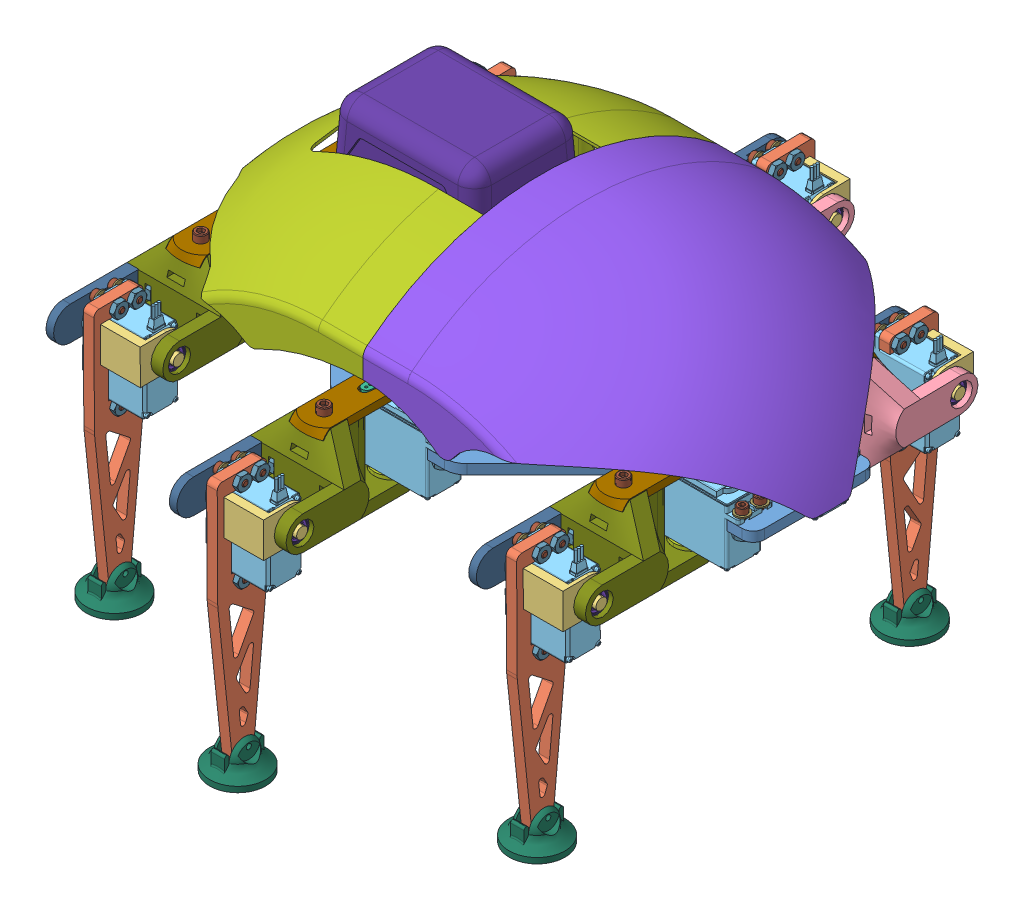
SolidWorks assembly Hexapod_NewBody, configuration Défaut. Lengths in mm.
Overall size (338.69 233.7 350.76).
398 component instances, 26 part files, 150 mates.
Components (placement in the parent):
- Body_V2-5: Body_V2 [Default] at (-310 -5.6 15) x (1 0 0) z (0 1 0) size (310 170 5.6)
- Leg_(Straight_Foot)-6: Leg_(Straight_Foot) [Default] at (-54.94 -26.67 -0.094) size (71.12 162.26 125.96)
  - Foot_(Straight)-1: Foot_(Straight) [Default] at (4.9357 4.6699 -91.3683) x (0.014203 -0.004158 0.99989) z (-0.999899 0 0.014203) size (28 145.4 6)
  - bearing_mount_foot-1: bearing_mount_foot [Default] at (4.8169 16.6428 -99.7277) x (-0.014203 0.004158 -0.99989) z (0.999899 0 -0.014203) size (25 20 29.5)
  - Joint-1: Joint [Défaut] at (35.768 26.4662 -54.7315) x (-0.014203 0 -0.999899) z (0 1 0) size (96.52 53.26 53.26)
  - hs-422-2: hs-422 [Défaut] at (5.1023 6.6131 -77.4551) x (-0.014203 0.004158 -0.99989) z (0.000059 0.999991 0.004158) size (19.81 42.09 58.23)
  - hs-422-3: hs-422 [Défaut] at (19.939 20.701 -19.812) x (0 0 1) z (-1 0 0) size (19.81 42.09 58.23)
  - hs-422_horn_straight-1: hs-422_horn_straight [Default] at (-16.9088 16.9412 -87.0065) x (0.014203 0 0.999899) z (0 1 0) size (33.93 4.93 8.79)
  - hs-422_horn_straight-2: hs-422_horn_straight [Default] at (9.652 42.5743 -9.906) x (-0.014203 0 -0.999899) z (-0.999899 0 0.014203) size (33.93 4.93 8.79)
  - Bearing_mount_leg-1: Bearing_mount_leg [Default] at (9.652 21 2.594) x (0 0 1) z (0 -1 0) size (35 20 30)
  - Bearing-1: Bearing [Default] at (9.652 -6.7498 -9.906) x (0.84763 0 0.530588) z (-0.530588 0 0.84763) size (13.87 4.75 13.87)
  - Bearing-2: Bearing [Default] at (32.2403 16.9412 -87.7047) x (0.007588 -0.845349 0.534161) z (-0.012007 -0.534214 -0.845264) size (13.87 4.75 13.87)
  - Joint_attachment_leg-1: Joint_attachment_leg [Défaut] at (35.768 26.4662 -54.7315) x (-0.014203 0 -0.999899) z (0 1 0) size (74.32 19.07 4.32)
  - Joint_attachment_foot-1: Joint_attachment_foot [Défaut] at (35.768 26.4662 -54.7315) x (-0.014203 0 -0.999899) z (0 1 0) size (64.08 6.7 19.07)
  - socket_1_2_6-32_with_washer-1: socket_1_2_6-32_with_washer [Défaut] at (43.4196 -14.698 -83.8589) x (0.999899 0 -0.014203) z (0.012271 -0.503597 0.863852) size (16.21 7.92 7.92)
    - socket head cap screw_ai-1: socket head cap screw_ai [HX-SHCS 0.138-32x0.5x0.5-N] at (-51.206 -1.62 2.0257) size (16.21 5.74 5.74)
    - flat washer type b narrow_ai-1: flat washer type b narrow_ai [Narrow FW 0.138] at (-46.888 -1.62 2.0257) size (0.81 7.92 7.92)
  - socket_1_2_6-32_with_washer-2: socket_1_2_6-32_with_washer [Défaut] at (43.2654 -19.0943 -94.7118) x (0.999899 0 -0.014203) z (0.000059 0.999991 0.004158) size (16.21 7.92 7.92)
    - socket head cap screw_ai-1: socket head cap screw_ai [HX-SHCS 0.138-32x0.5x0.5-N] at (-51.206 -1.62 2.0257) size (16.21 5.74 5.74)
    - flat washer type b narrow_ai-1: flat washer type b narrow_ai [Narrow FW 0.138] at (-46.888 -1.62 2.0257) size (0.81 7.92 7.92)
  - socket_1_2_6-32_with_washer-3: socket_1_2_6-32_with_washer [Défaut] at (43.4489 27.9623 -81.7931) x (0.999899 0 -0.014203) z (-0.012271 0.503597 -0.863852) size (16.21 7.92 7.92)
    - socket head cap screw_ai-1: socket head cap screw_ai [HX-SHCS 0.138-32x0.5x0.5-N] at (-51.206 -1.62 2.0257) size (16.21 5.74 5.74)
    - flat washer type b narrow_ai-1: flat washer type b narrow_ai [Narrow FW 0.138] at (-46.888 -1.62 2.0257) size (0.81 7.92 7.92)
  - socket_1_2_6-32_with_washer-4: socket_1_2_6-32_with_washer [Défaut] at (43.3046 28.0045 -91.952) x (0.999899 0 -0.014203) z (-0.012271 0.503597 -0.863852) size (16.21 7.92 7.92)
    - socket head cap screw_ai-1: socket head cap screw_ai [HX-SHCS 0.138-32x0.5x0.5-N] at (-51.206 -1.62 2.0257) size (16.21 5.74 5.74)
    - flat washer type b narrow_ai-1: flat washer type b narrow_ai [Narrow FW 0.138] at (-46.888 -1.62 2.0257) size (0.81 7.92 7.92)
  - socket button head cap screw_ai-2: socket button head cap screw_ai [SBHCSCREW 0.112-40x0.25-HX-N] at (-19.9057 16.9412 -86.964) x (0.999899 0 -0.014203) z (-0.007102 0.866025 -0.49995) size (7.85 5.41 5.41)
  - socket button head cap screw_ai-3: socket button head cap screw_ai [SBHCSCREW 0.112-40x0.25-HX-N] at (9.652 45.5715 -9.906) x (0 -1 0) z (0.87304 0 0.487649) size (7.85 5.41 5.41)
  - machine screw nut hex_ai-7: machine screw nut hex_ai [MSHXNUT 0.138-32-D-N] at (5.0634 -17.1176 -82.3797) x (0.01233 0.496395 0.868009) z (-0.999899 0 0.014203) size (7.92 9.15 2.9)
  - machine screw nut hex_ai-8: machine screw nut hex_ai [MSHXNUT 0.138-32-D-N] at (4.9191 -17.0754 -92.5386) x (-0.012271 0.503597 -0.863852) z (-0.999899 0 0.014203) size (7.92 9.15 2.9)
  - machine screw nut hex_ai-9: machine screw nut hex_ai [MSHXNUT 0.138-32-D-N] at (5.0662 30.382 -82.1822) x (0.000059 0.999991 0.004158) z (-0.999899 0 0.014203) size (7.92 9.15 2.9)
  - machine screw nut hex_ai-10: machine screw nut hex_ai [MSHXNUT 0.138-32-D-N] at (4.9219 30.4242 -92.3411) x (0.000059 0.999991 0.004158) z (-0.999899 0 0.014203) size (7.92 9.15 2.9)
  - socket head cap screw_ai-1: socket head cap screw_ai [HX-SHCS 0.164-32x0.5x0.5-N] at (9.1052 47.8568 -48.4) x (0 -1 0) z (0.014203 0 0.999899) size (16.87 6.86 6.86)
  - socket head cap screw_ai-2: socket head cap screw_ai [HX-SHCS 0.164-32x0.5x0.5-N] at (-21.967 16.9412 -59.205) x (0.999899 0 -0.014203) z (0.014203 0 0.999899) size (16.87 6.86 6.86)
  - machine screw nut hex_ai-11: machine screw nut hex_ai [MSHXNUT 0.164-32-D-N] at (9.1052 33.127 -48.4) x (0.87304 0 0.487649) z (0 1 0) size (8.74 10.09 3.3)
  - machine screw nut hex_ai-12: machine screw nut hex_ai [MSHXNUT 0.164-32-D-N] at (-7.2387 16.9412 -59.4142) x (0.014203 0 0.999899) z (-0.999899 0 0.014203) size (8.74 10.09 3.3)
  - socket head cap screw_ai-3: socket head cap screw_ai [HX-SHCS 0.112-40x0.5x0.5-N] at (-4.0273 11.7048 -99.6226) x (0.999899 0 -0.014203) z (0.014203 -0.004158 0.99989) size (15.54 4.65 4.65)
  - socket head cap screw_ai-4: socket head cap screw_ai [HX-SHCS 0.112-40x0.5x0.5-N] at (-4.0267 21.7048 -99.5811) x (0.999899 0 -0.014203) z (-0.014203 0.004158 -0.99989) size (15.54 4.65 4.65)
  - socket_1_2_6-32_with_washer-5: socket_1_2_6-32_with_washer [Défaut] at (-3.4199 -17.7034 -7.3903) x (0 -1 0) z (0.5 0 0.866025) size (16.21 7.92 7.92)
    - socket head cap screw_ai-1: socket head cap screw_ai [HX-SHCS 0.138-32x0.5x0.5-N] at (-51.206 -1.62 2.0257) size (16.21 5.74 5.74)
    - flat washer type b narrow_ai-1: flat washer type b narrow_ai [Narrow FW 0.138] at (-46.888 -1.62 2.0257) size (0.81 7.92 7.92)
  - socket_1_2_6-32_with_washer-6: socket_1_2_6-32_with_washer [Défaut] at (44.0781 -17.7034 -17.5503) x (0 -1 0) z (0.5 0 0.866025) size (16.21 7.92 7.92)
    - socket head cap screw_ai-1: socket head cap screw_ai [HX-SHCS 0.138-32x0.5x0.5-N] at (-51.206 -1.62 2.0257) size (16.21 5.74 5.74)
    - flat washer type b narrow_ai-1: flat washer type b narrow_ai [Narrow FW 0.138] at (-46.888 -1.62 2.0257) size (0.81 7.92 7.92)
  - socket_1_2_6-32_with_washer-7: socket_1_2_6-32_with_washer [Défaut] at (-3.4199 -17.7034 -17.5503) x (0 -1 0) z (0.5 0 0.866025) size (16.21 7.92 7.92)
    - socket head cap screw_ai-1: socket head cap screw_ai [HX-SHCS 0.138-32x0.5x0.5-N] at (-51.206 -1.62 2.0257) size (16.21 5.74 5.74)
    - flat washer type b narrow_ai-1: flat washer type b narrow_ai [Narrow FW 0.138] at (-46.888 -1.62 2.0257) size (0.81 7.92 7.92)
  - socket_1_2_6-32_with_washer-8: socket_1_2_6-32_with_washer [Défaut] at (44.0781 -17.7034 -7.3903) x (0 -1 0) z (0.5 0 0.866025) size (16.21 7.92 7.92)
    - socket head cap screw_ai-1: socket head cap screw_ai [HX-SHCS 0.138-32x0.5x0.5-N] at (-51.206 -1.62 2.0257) size (16.21 5.74 5.74)
    - flat washer type b narrow_ai-1: flat washer type b narrow_ai [Narrow FW 0.138] at (-46.888 -1.62 2.0257) size (0.81 7.92 7.92)
  - Slippers-1: Slippers [Default] at (1.9298 -111.2299 -91.7597) x (0.999899 0 -0.014203) z (0.014203 0 0.999899) size (35.48 18.25 37.71)
- Leg_(Straight_Foot)-7: Leg_(Straight_Foot) [Default] at (-294.94 -26.67 -0.094) size (71.12 162.26 125.96)
  - Foot_(Straight)-1: Foot_(Straight) [Default] at (4.9357 4.6699 -91.3683) x (0.014203 -0.004158 0.99989) z (-0.999899 0 0.014203) size (28 145.4 6)
  - bearing_mount_foot-1: bearing_mount_foot [Default] at (4.8169 16.6428 -99.7277) x (-0.014203 0.004158 -0.99989) z (0.999899 0 -0.014203) size (25 20 29.5)
  - Joint-1: Joint [Défaut] at (35.768 26.4662 -54.7315) x (-0.014203 0 -0.999899) z (0 1 0) size (96.52 53.26 53.26)
  - hs-422-2: hs-422 [Défaut] at (5.1023 6.6131 -77.4551) x (-0.014203 0.004158 -0.99989) z (0.000059 0.999991 0.004158) size (19.81 42.09 58.23)
  - hs-422-3: hs-422 [Défaut] at (19.939 20.701 -19.812) x (0 0 1) z (-1 0 0) size (19.81 42.09 58.23)
  - hs-422_horn_straight-1: hs-422_horn_straight [Default] at (-16.9088 16.9412 -87.0065) x (0.014203 0 0.999899) z (0 1 0) size (33.93 4.93 8.79)
  - hs-422_horn_straight-2: hs-422_horn_straight [Default] at (9.652 42.5743 -9.906) x (-0.014203 0 -0.999899) z (-0.999899 0 0.014203) size (33.93 4.93 8.79)
  - Bearing_mount_leg-1: Bearing_mount_leg [Default] at (9.652 21 2.594) x (0 0 1) z (0 -1 0) size (35 20 30)
  - Bearing-1: Bearing [Default] at (9.652 -6.7498 -9.906) x (0.84763 0 0.530588) z (-0.530588 0 0.84763) size (13.87 4.75 13.87)
  - Bearing-2: Bearing [Default] at (32.2403 16.9412 -87.7047) x (0.007588 -0.845349 0.534161) z (-0.012007 -0.534214 -0.845264) size (13.87 4.75 13.87)
  - Joint_attachment_leg-1: Joint_attachment_leg [Défaut] at (35.768 26.4662 -54.7315) x (-0.014203 0 -0.999899) z (0 1 0) size (74.32 19.07 4.32)
  - Joint_attachment_foot-1: Joint_attachment_foot [Défaut] at (35.768 26.4662 -54.7315) x (-0.014203 0 -0.999899) z (0 1 0) size (64.08 6.7 19.07)
  - socket_1_2_6-32_with_washer-1: socket_1_2_6-32_with_washer [Défaut] at (43.4196 -14.698 -83.8589) x (0.999899 0 -0.014203) z (0.012271 -0.503597 0.863852) size (16.21 7.92 7.92)
    - socket head cap screw_ai-1: socket head cap screw_ai [HX-SHCS 0.138-32x0.5x0.5-N] at (-51.206 -1.62 2.0257) size (16.21 5.74 5.74)
    - flat washer type b narrow_ai-1: flat washer type b narrow_ai [Narrow FW 0.138] at (-46.888 -1.62 2.0257) size (0.81 7.92 7.92)
  - socket_1_2_6-32_with_washer-2: socket_1_2_6-32_with_washer [Défaut] at (43.2654 -19.0943 -94.7118) x (0.999899 0 -0.014203) z (0.000059 0.999991 0.004158) size (16.21 7.92 7.92)
    - socket head cap screw_ai-1: socket head cap screw_ai [HX-SHCS 0.138-32x0.5x0.5-N] at (-51.206 -1.62 2.0257) size (16.21 5.74 5.74)
    - flat washer type b narrow_ai-1: flat washer type b narrow_ai [Narrow FW 0.138] at (-46.888 -1.62 2.0257) size (0.81 7.92 7.92)
  - socket_1_2_6-32_with_washer-3: socket_1_2_6-32_with_washer [Défaut] at (43.4489 27.9623 -81.7931) x (0.999899 0 -0.014203) z (-0.012271 0.503597 -0.863852) size (16.21 7.92 7.92)
    - socket head cap screw_ai-1: socket head cap screw_ai [HX-SHCS 0.138-32x0.5x0.5-N] at (-51.206 -1.62 2.0257) size (16.21 5.74 5.74)
    - flat washer type b narrow_ai-1: flat washer type b narrow_ai [Narrow FW 0.138] at (-46.888 -1.62 2.0257) size (0.81 7.92 7.92)
  - socket_1_2_6-32_with_washer-4: socket_1_2_6-32_with_washer [Défaut] at (43.3046 28.0045 -91.952) x (0.999899 0 -0.014203) z (-0.012271 0.503597 -0.863852) size (16.21 7.92 7.92)
    - socket head cap screw_ai-1: socket head cap screw_ai [HX-SHCS 0.138-32x0.5x0.5-N] at (-51.206 -1.62 2.0257) size (16.21 5.74 5.74)
    - flat washer type b narrow_ai-1: flat washer type b narrow_ai [Narrow FW 0.138] at (-46.888 -1.62 2.0257) size (0.81 7.92 7.92)
  - socket button head cap screw_ai-2: socket button head cap screw_ai [SBHCSCREW 0.112-40x0.25-HX-N] at (-19.9057 16.9412 -86.964) x (0.999899 0 -0.014203) z (-0.007102 0.866025 -0.49995) size (7.85 5.41 5.41)
  - socket button head cap screw_ai-3: socket button head cap screw_ai [SBHCSCREW 0.112-40x0.25-HX-N] at (9.652 45.5715 -9.906) x (0 -1 0) z (0.87304 0 0.487649) size (7.85 5.41 5.41)
  - machine screw nut hex_ai-7: machine screw nut hex_ai [MSHXNUT 0.138-32-D-N] at (5.0634 -17.1176 -82.3797) x (0.01233 0.496395 0.868009) z (-0.999899 0 0.014203) size (7.92 9.15 2.9)
  - machine screw nut hex_ai-8: machine screw nut hex_ai [MSHXNUT 0.138-32-D-N] at (4.9191 -17.0754 -92.5386) x (-0.012271 0.503597 -0.863852) z (-0.999899 0 0.014203) size (7.92 9.15 2.9)
  - machine screw nut hex_ai-9: machine screw nut hex_ai [MSHXNUT 0.138-32-D-N] at (5.0662 30.382 -82.1822) x (0.000059 0.999991 0.004158) z (-0.999899 0 0.014203) size (7.92 9.15 2.9)
  - machine screw nut hex_ai-10: machine screw nut hex_ai [MSHXNUT 0.138-32-D-N] at (4.9219 30.4242 -92.3411) x (0.000059 0.999991 0.004158) z (-0.999899 0 0.014203) size (7.92 9.15 2.9)
  - socket head cap screw_ai-1: socket head cap screw_ai [HX-SHCS 0.164-32x0.5x0.5-N] at (9.1052 47.8568 -48.4) x (0 -1 0) z (0.014203 0 0.999899) size (16.87 6.86 6.86)
  - socket head cap screw_ai-2: socket head cap screw_ai [HX-SHCS 0.164-32x0.5x0.5-N] at (-21.967 16.9412 -59.205) x (0.999899 0 -0.014203) z (0.014203 0 0.999899) size (16.87 6.86 6.86)
  - machine screw nut hex_ai-11: machine screw nut hex_ai [MSHXNUT 0.164-32-D-N] at (9.1052 33.127 -48.4) x (0.87304 0 0.487649) z (0 1 0) size (8.74 10.09 3.3)
  - machine screw nut hex_ai-12: machine screw nut hex_ai [MSHXNUT 0.164-32-D-N] at (-7.2387 16.9412 -59.4142) x (0.014203 0 0.999899) z (-0.999899 0 0.014203) size (8.74 10.09 3.3)
  - socket head cap screw_ai-3: socket head cap screw_ai [HX-SHCS 0.112-40x0.5x0.5-N] at (-4.0273 11.7048 -99.6226) x (0.999899 0 -0.014203) z (0.014203 -0.004158 0.99989) size (15.54 4.65 4.65)
  - socket head cap screw_ai-4: socket head cap screw_ai [HX-SHCS 0.112-40x0.5x0.5-N] at (-4.0267 21.7048 -99.5811) x (0.999899 0 -0.014203) z (-0.014203 0.004158 -0.99989) size (15.54 4.65 4.65)
  - socket_1_2_6-32_with_washer-5: socket_1_2_6-32_with_washer [Défaut] at (-3.4199 -17.7034 -7.3903) x (0 -1 0) z (0.5 0 0.866025) size (16.21 7.92 7.92)
    - socket head cap screw_ai-1: socket head cap screw_ai [HX-SHCS 0.138-32x0.5x0.5-N] at (-51.206 -1.62 2.0257) size (16.21 5.74 5.74)
    - flat washer type b narrow_ai-1: flat washer type b narrow_ai [Narrow FW 0.138] at (-46.888 -1.62 2.0257) size (0.81 7.92 7.92)
  - socket_1_2_6-32_with_washer-6: socket_1_2_6-32_with_washer [Défaut] at (44.0781 -17.7034 -17.5503) x (0 -1 0) z (0.5 0 0.866025) size (16.21 7.92 7.92)
    - socket head cap screw_ai-1: socket head cap screw_ai [HX-SHCS 0.138-32x0.5x0.5-N] at (-51.206 -1.62 2.0257) size (16.21 5.74 5.74)
    - flat washer type b narrow_ai-1: flat washer type b narrow_ai [Narrow FW 0.138] at (-46.888 -1.62 2.0257) size (0.81 7.92 7.92)
  - socket_1_2_6-32_with_washer-7: socket_1_2_6-32_with_washer [Défaut] at (-3.4199 -17.7034 -17.5503) x (0 -1 0) z (0.5 0 0.866025) size (16.21 7.92 7.92)
    - socket head cap screw_ai-1: socket head cap screw_ai [HX-SHCS 0.138-32x0.5x0.5-N] at (-51.206 -1.62 2.0257) size (16.21 5.74 5.74)
    - flat washer type b narrow_ai-1: flat washer type b narrow_ai [Narrow FW 0.138] at (-46.888 -1.62 2.0257) size (0.81 7.92 7.92)
  - socket_1_2_6-32_with_washer-8: socket_1_2_6-32_with_washer [Défaut] at (44.0781 -17.7034 -7.3903) x (0 -1 0) z (0.5 0 0.866025) size (16.21 7.92 7.92)
    - socket head cap screw_ai-1: socket head cap screw_ai [HX-SHCS 0.138-32x0.5x0.5-N] at (-51.206 -1.62 2.0257) size (16.21 5.74 5.74)
    - flat washer type b narrow_ai-1: flat washer type b narrow_ai [Narrow FW 0.138] at (-46.888 -1.62 2.0257) size (0.81 7.92 7.92)
  - Slippers-1: Slippers [Default] at (1.9298 -111.2299 -91.7597) x (0.999899 0 -0.014203) z (0.014203 0 0.999899) size (35.48 18.25 37.71)
- Leg_(Straight_Foot)-8: Leg_(Straight_Foot) [Default] at (-174.94 -26.67 -50.094) size (71.12 162.26 125.96)
  - Foot_(Straight)-1: Foot_(Straight) [Default] at (4.9357 4.6699 -91.3683) x (0.014203 -0.004158 0.99989) z (-0.999899 0 0.014203) size (28 145.4 6)
  - bearing_mount_foot-1: bearing_mount_foot [Default] at (4.8169 16.6428 -99.7277) x (-0.014203 0.004158 -0.99989) z (0.999899 0 -0.014203) size (25 20 29.5)
  - Joint-1: Joint [Défaut] at (35.768 26.4662 -54.7315) x (-0.014203 0 -0.999899) z (0 1 0) size (96.52 53.26 53.26)
  - hs-422-2: hs-422 [Défaut] at (5.1023 6.6131 -77.4551) x (-0.014203 0.004158 -0.99989) z (0.000059 0.999991 0.004158) size (19.81 42.09 58.23)
  - hs-422-3: hs-422 [Défaut] at (19.939 20.701 -19.812) x (0 0 1) z (-1 0 0) size (19.81 42.09 58.23)
  - hs-422_horn_straight-1: hs-422_horn_straight [Default] at (-16.9088 16.9412 -87.0065) x (0.014203 0 0.999899) z (0 1 0) size (33.93 4.93 8.79)
  - hs-422_horn_straight-2: hs-422_horn_straight [Default] at (9.652 42.5743 -9.906) x (-0.014203 0 -0.999899) z (-0.999899 0 0.014203) size (33.93 4.93 8.79)
  - Bearing_mount_leg-1: Bearing_mount_leg [Default] at (9.652 21 2.594) x (0 0 1) z (0 -1 0) size (35 20 30)
  - Bearing-1: Bearing [Default] at (9.652 -6.7498 -9.906) x (0.84763 0 0.530588) z (-0.530588 0 0.84763) size (13.87 4.75 13.87)
  - Bearing-2: Bearing [Default] at (32.2403 16.9412 -87.7047) x (0.007588 -0.845349 0.534161) z (-0.012007 -0.534214 -0.845264) size (13.87 4.75 13.87)
  - Joint_attachment_leg-1: Joint_attachment_leg [Défaut] at (35.768 26.4662 -54.7315) x (-0.014203 0 -0.999899) z (0 1 0) size (74.32 19.07 4.32)
  - Joint_attachment_foot-1: Joint_attachment_foot [Défaut] at (35.768 26.4662 -54.7315) x (-0.014203 0 -0.999899) z (0 1 0) size (64.08 6.7 19.07)
  - socket_1_2_6-32_with_washer-1: socket_1_2_6-32_with_washer [Défaut] at (43.4196 -14.698 -83.8589) x (0.999899 0 -0.014203) z (0.012271 -0.503597 0.863852) size (16.21 7.92 7.92)
    - socket head cap screw_ai-1: socket head cap screw_ai [HX-SHCS 0.138-32x0.5x0.5-N] at (-51.206 -1.62 2.0257) size (16.21 5.74 5.74)
    - flat washer type b narrow_ai-1: flat washer type b narrow_ai [Narrow FW 0.138] at (-46.888 -1.62 2.0257) size (0.81 7.92 7.92)
  - socket_1_2_6-32_with_washer-2: socket_1_2_6-32_with_washer [Défaut] at (43.2654 -19.0943 -94.7118) x (0.999899 0 -0.014203) z (0.000059 0.999991 0.004158) size (16.21 7.92 7.92)
    - socket head cap screw_ai-1: socket head cap screw_ai [HX-SHCS 0.138-32x0.5x0.5-N] at (-51.206 -1.62 2.0257) size (16.21 5.74 5.74)
    - flat washer type b narrow_ai-1: flat washer type b narrow_ai [Narrow FW 0.138] at (-46.888 -1.62 2.0257) size (0.81 7.92 7.92)
  - socket_1_2_6-32_with_washer-3: socket_1_2_6-32_with_washer [Défaut] at (43.4489 27.9623 -81.7931) x (0.999899 0 -0.014203) z (-0.012271 0.503597 -0.863852) size (16.21 7.92 7.92)
    - socket head cap screw_ai-1: socket head cap screw_ai [HX-SHCS 0.138-32x0.5x0.5-N] at (-51.206 -1.62 2.0257) size (16.21 5.74 5.74)
    - flat washer type b narrow_ai-1: flat washer type b narrow_ai [Narrow FW 0.138] at (-46.888 -1.62 2.0257) size (0.81 7.92 7.92)
  - socket_1_2_6-32_with_washer-4: socket_1_2_6-32_with_washer [Défaut] at (43.3046 28.0045 -91.952) x (0.999899 0 -0.014203) z (-0.012271 0.503597 -0.863852) size (16.21 7.92 7.92)
    - socket head cap screw_ai-1: socket head cap screw_ai [HX-SHCS 0.138-32x0.5x0.5-N] at (-51.206 -1.62 2.0257) size (16.21 5.74 5.74)
    - flat washer type b narrow_ai-1: flat washer type b narrow_ai [Narrow FW 0.138] at (-46.888 -1.62 2.0257) size (0.81 7.92 7.92)
  - socket button head cap screw_ai-2: socket button head cap screw_ai [SBHCSCREW 0.112-40x0.25-HX-N] at (-19.9057 16.9412 -86.964) x (0.999899 0 -0.014203) z (-0.007102 0.866025 -0.49995) size (7.85 5.41 5.41)
  - socket button head cap screw_ai-3: socket button head cap screw_ai [SBHCSCREW 0.112-40x0.25-HX-N] at (9.652 45.5715 -9.906) x (0 -1 0) z (0.87304 0 0.487649) size (7.85 5.41 5.41)
  - machine screw nut hex_ai-7: machine screw nut hex_ai [MSHXNUT 0.138-32-D-N] at (5.0634 -17.1176 -82.3797) x (0.01233 0.496395 0.868009) z (-0.999899 0 0.014203) size (7.92 9.15 2.9)
  - machine screw nut hex_ai-8: machine screw nut hex_ai [MSHXNUT 0.138-32-D-N] at (4.9191 -17.0754 -92.5386) x (-0.012271 0.503597 -0.863852) z (-0.999899 0 0.014203) size (7.92 9.15 2.9)
  - machine screw nut hex_ai-9: machine screw nut hex_ai [MSHXNUT 0.138-32-D-N] at (5.0662 30.382 -82.1822) x (0.000059 0.999991 0.004158) z (-0.999899 0 0.014203) size (7.92 9.15 2.9)
  - machine screw nut hex_ai-10: machine screw nut hex_ai [MSHXNUT 0.138-32-D-N] at (4.9219 30.4242 -92.3411) x (0.000059 0.999991 0.004158) z (-0.999899 0 0.014203) size (7.92 9.15 2.9)
  - socket head cap screw_ai-1: socket head cap screw_ai [HX-SHCS 0.164-32x0.5x0.5-N] at (9.1052 47.8568 -48.4) x (0 -1 0) z (0.014203 0 0.999899) size (16.87 6.86 6.86)
  - socket head cap screw_ai-2: socket head cap screw_ai [HX-SHCS 0.164-32x0.5x0.5-N] at (-21.967 16.9412 -59.205) x (0.999899 0 -0.014203) z (0.014203 0 0.999899) size (16.87 6.86 6.86)
  - machine screw nut hex_ai-11: machine screw nut hex_ai [MSHXNUT 0.164-32-D-N] at (9.1052 33.127 -48.4) x (0.87304 0 0.487649) z (0 1 0) size (8.74 10.09 3.3)
  - machine screw nut hex_ai-12: machine screw nut hex_ai [MSHXNUT 0.164-32-D-N] at (-7.2387 16.9412 -59.4142) x (0.014203 0 0.999899) z (-0.999899 0 0.014203) size (8.74 10.09 3.3)
  - socket head cap screw_ai-3: socket head cap screw_ai [HX-SHCS 0.112-40x0.5x0.5-N] at (-4.0273 11.7048 -99.6226) x (0.999899 0 -0.014203) z (0.014203 -0.004158 0.99989) size (15.54 4.65 4.65)
  - socket head cap screw_ai-4: socket head cap screw_ai [HX-SHCS 0.112-40x0.5x0.5-N] at (-4.0267 21.7048 -99.5811) x (0.999899 0 -0.014203) z (-0.014203 0.004158 -0.99989) size (15.54 4.65 4.65)
  - socket_1_2_6-32_with_washer-5: socket_1_2_6-32_with_washer [Défaut] at (-3.4199 -17.7034 -7.3903) x (0 -1 0) z (0.5 0 0.866025) size (16.21 7.92 7.92)
    - socket head cap screw_ai-1: socket head cap screw_ai [HX-SHCS 0.138-32x0.5x0.5-N] at (-51.206 -1.62 2.0257) size (16.21 5.74 5.74)
    - flat washer type b narrow_ai-1: flat washer type b narrow_ai [Narrow FW 0.138] at (-46.888 -1.62 2.0257) size (0.81 7.92 7.92)
  - socket_1_2_6-32_with_washer-6: socket_1_2_6-32_with_washer [Défaut] at (44.0781 -17.7034 -17.5503) x (0 -1 0) z (0.5 0 0.866025) size (16.21 7.92 7.92)
    - socket head cap screw_ai-1: socket head cap screw_ai [HX-SHCS 0.138-32x0.5x0.5-N] at (-51.206 -1.62 2.0257) size (16.21 5.74 5.74)
    - flat washer type b narrow_ai-1: flat washer type b narrow_ai [Narrow FW 0.138] at (-46.888 -1.62 2.0257) size (0.81 7.92 7.92)
  - socket_1_2_6-32_with_washer-7: socket_1_2_6-32_with_washer [Défaut] at (-3.4199 -17.7034 -17.5503) x (0 -1 0) z (0.5 0 0.866025) size (16.21 7.92 7.92)
    - socket head cap screw_ai-1: socket head cap screw_ai [HX-SHCS 0.138-32x0.5x0.5-N] at (-51.206 -1.62 2.0257) size (16.21 5.74 5.74)
    - flat washer type b narrow_ai-1: flat washer type b narrow_ai [Narrow FW 0.138] at (-46.888 -1.62 2.0257) size (0.81 7.92 7.92)
  - socket_1_2_6-32_with_washer-8: socket_1_2_6-32_with_washer [Défaut] at (44.0781 -17.7034 -7.3903) x (0 -1 0) z (0.5 0 0.866025) size (16.21 7.92 7.92)
    - socket head cap screw_ai-1: socket head cap screw_ai [HX-SHCS 0.138-32x0.5x0.5-N] at (-51.206 -1.62 2.0257) size (16.21 5.74 5.74)
    - flat washer type b narrow_ai-1: flat washer type b narrow_ai [Narrow FW 0.138] at (-46.888 -1.62 2.0257) size (0.81 7.92 7.92)
  - Slippers-1: Slippers [Default] at (1.9298 -111.2299 -91.7597) x (0.999899 0 -0.014203) z (0.014203 0 0.999899) size (35.48 18.25 37.71)
- Leg_(Straight_Foot)_(Mirror)-4: Leg_(Straight_Foot)_(Mirror) [Default] at (-294.94 -26.67 49.906) size (70.34 162.3 124.8)
  - Joint_(Mirror)-1: Joint_(Mirror) [Défaut] at (36.4933 -51.1276 34.4889) x (0.002055 0 0.999998) z (0 -1 0) size (96.52 53.26 53.26)
  - hs-422-3: hs-422 [Défaut] at (19.939 20.701 -19.812) x (0 0 1) z (-1 0 0) size (19.81 42.09 58.23)
  - hs-422_horn_straight-2: hs-422_horn_straight [Default] at (9.652 42.5743 -9.906) x (0.002055 0 0.999998) z (0.999998 0 -0.002055) size (33.93 4.93 8.79)
  - Bearing_mount_leg-1: Bearing_mount_leg [Default] at (9.652 21 -22.406) x (0 0 -1) z (0 -1 0) size (35 20 30)
  - Bearing-1: Bearing [Default] at (9.652 -6.7498 -9.906) x (0.266287 0 0.963894) z (-0.963894 0 0.266287) size (13.87 4.75 13.87)
  - Joint_attachment_leg-1: Joint_attachment_leg [Défaut] at (-17.0066 26.5024 34.5989) x (0.002055 0 0.999998) z (0 1 0) size (74.32 19.07 4.32)
  - bearing_mount_foot-2: bearing_mount_foot [Default] at (6.7141 17.2663 79.9818) x (0.002055 -0.004919 0.999986) z (0.999998 0 -0.002055) size (25 20 29.5)
  - Bearing-3: Bearing [Default] at (29.1886 16.9774 67.524) x (-0.001098 -0.845349 -0.534213) z (0.001738 -0.534214 0.845347) size (13.87 4.75 13.87)
  - hs-422-4: hs-422 [Défaut] at (6.0779 6.6418 77.4268) x (-0.002055 0.004919 -0.999986) z (0.00001 0.999988 0.004919) size (19.81 42.09 58.23)
  - hs-422_horn_straight-3: hs-422_horn_straight [Default] at (-15.8156 16.9774 67.6165) x (-0.002055 0 -0.999998) z (0 -1 0) size (33.93 4.93 8.79)
  - Foot_(Straight)-2: Foot_(Straight) [Default] at (0.0967 4.6719 71.5233) x (-0.002055 0.004919 -0.999986) z (0.999998 0 -0.002055) size (28 145.4 6)
  - Joint_attachment_foot-2: Joint_attachment_foot [Défaut] at (36.4933 7.4524 34.4889) x (0.002055 0 0.999998) z (0 -1 0) size (64.08 6.7 19.07)
  - socket button head cap screw_ai-1: socket button head cap screw_ai [SBHCSCREW 0.138-32x0.25-HX-N] at (-19.1684 16.9774 67.6234) x (0.999998 0 -0.002055) z (0.002055 0 0.999998) size (8.2 6.65 6.65)
  - socket button head cap screw_ai-2: socket button head cap screw_ai [SBHCSCREW 0.138-32x0.25-HX-N] at (9.652 45.9271 -9.906) x (0 -1 0) z (-0.864996 0 0.501779) size (8.2 6.65 6.65)
  - socket head cap screw_ai-1: socket head cap screw_ai [HX-SHCS 0.112-40x0.5x0.5-N] at (-2.7306 21.6303 80.0227) x (0.999998 0 -0.002055) z (0.001019 -0.868474 0.495733) size (15.54 4.65 4.65)
  - socket head cap screw_ai-2: socket head cap screw_ai [HX-SHCS 0.112-40x0.5x0.5-N] at (-2.7307 11.6304 79.9735) x (0.999998 0 -0.002055) z (0.001036 0.863555 0.504253) size (15.54 4.65 4.65)
  - socket head cap screw_ai-3: socket head cap screw_ai [HX-SHCS 0.164-32x0.5x0.5-N] at (-21.1613 16.9774 39.9006) x (0.999998 0 -0.002055) z (0.001028 0.866025 0.499999) size (16.87 6.86 6.86)
  - socket head cap screw_ai-4: socket head cap screw_ai [HX-SHCS 0.164-32x0.5x0.5-N] at (9.7311 47.893 28.5918) x (0 -1 0) z (0.002055 0 0.999998) size (16.87 6.86 6.86)
  - socket_1_2_6-32_with_washer-1: socket_1_2_6-32_with_washer [Défaut] at (44.4497 32.8866 61.5465) x (0.999998 0 -0.002055) z (0.001775 -0.504254 0.863554) size (16.21 7.92 7.92)
    - socket head cap screw_ai-1: socket head cap screw_ai [HX-SHCS 0.138-32x0.5x0.5-N] at (-51.206 -1.62 2.0257) size (16.21 5.74 5.74)
    - flat washer type b narrow_ai-1: flat washer type b narrow_ai [Narrow FW 0.138] at (-46.888 -1.62 2.0257) size (0.81 7.92 7.92)
  - socket_1_2_6-32_with_washer-2: socket_1_2_6-32_with_washer [Défaut] at (44.4545 -15.0155 63.8752) x (0.999998 0 -0.002055) z (-0.00001 -0.999988 -0.004919) size (16.21 7.92 7.92)
    - socket head cap screw_ai-1: socket head cap screw_ai [HX-SHCS 0.138-32x0.5x0.5-N] at (-51.206 -1.62 2.0257) size (16.21 5.74 5.74)
    - flat washer type b narrow_ai-1: flat washer type b narrow_ai [Narrow FW 0.138] at (-46.888 -1.62 2.0257) size (0.81 7.92 7.92)
  - socket_1_2_6-32_with_washer-3: socket_1_2_6-32_with_washer [Défaut] at (44.4701 -14.6628 71.4727) x (0.999998 0 -0.002055) z (0.001775 -0.504254 0.863554) size (16.21 7.92 7.92)
    - socket head cap screw_ai-1: socket head cap screw_ai [HX-SHCS 0.138-32x0.5x0.5-N] at (-51.206 -1.62 2.0257) size (16.21 5.74 5.74)
    - flat washer type b narrow_ai-1: flat washer type b narrow_ai [Narrow FW 0.138] at (-46.888 -1.62 2.0257) size (0.81 7.92 7.92)
  - socket_1_2_6-32_with_washer-4: socket_1_2_6-32_with_washer [Défaut] at (44.4706 32.8366 71.7064) x (0.999998 0 -0.002055) z (0.001775 -0.504254 0.863554) size (16.21 7.92 7.92)
    - socket head cap screw_ai-1: socket head cap screw_ai [HX-SHCS 0.138-32x0.5x0.5-N] at (-51.206 -1.62 2.0257) size (16.21 5.74 5.74)
    - flat washer type b narrow_ai-1: flat washer type b narrow_ai [Narrow FW 0.138] at (-46.888 -1.62 2.0257) size (0.81 7.92 7.92)
  - machine screw nut hex_ai-4: machine screw nut hex_ai [MSHXNUT 0.138-32-D-N] at (6.0779 -17.0332 62.3241) x (-0.001785 -0.495734 -0.868473) z (-0.999998 0 0.002055) size (7.92 9.15 2.9)
  - machine screw nut hex_ai-7: machine screw nut hex_ai [MSHXNUT 0.138-32-D-N] at (8.9943 -17.0832 72.478) x (-0.001775 0.504254 -0.863554) z (0.999998 0 -0.002055) size (7.92 9.15 2.9)
  - machine screw nut hex_ai-8: machine screw nut hex_ai [MSHXNUT 0.138-32-D-N] at (8.9739 30.4662 62.5518) x (0.00001 0.999988 0.004919) z (0.999998 0 -0.002055) size (7.92 9.15 2.9)
  - machine screw nut hex_ai-9: machine screw nut hex_ai [MSHXNUT 0.138-32-D-N] at (6.0992 30.4162 72.7176) x (-0.001785 -0.495734 -0.868473) z (-0.999998 0 0.002055) size (7.92 9.15 2.9)
  - socket_1_2_6-32_with_washer-5: socket_1_2_6-32_with_washer [Défaut] at (-3.4199 -17.7034 -7.3903) x (0 -1 0) z (0.5 0 0.866025) size (16.21 7.92 7.92)
    - socket head cap screw_ai-1: socket head cap screw_ai [HX-SHCS 0.138-32x0.5x0.5-N] at (-51.206 -1.62 2.0257) size (16.21 5.74 5.74)
    - flat washer type b narrow_ai-1: flat washer type b narrow_ai [Narrow FW 0.138] at (-46.888 -1.62 2.0257) size (0.81 7.92 7.92)
  - socket head cap screw_ai-5: socket head cap screw_ai [HX-SHCS 0.138-32x0.5x0.5-N] at (-3.81 33.5026 -14.986) x (0 -1 0) z (-1 0 0) size (16.21 5.74 5.74)
  - flat washer type b narrow_ai-1: flat washer type b narrow_ai [Narrow FW 0.138] at (-3.81 29.1846 -14.986) x (0 -1 0) z (0.546944 0 -0.837169) size (0.81 7.92 7.92)
  - socket head cap screw_ai-6: socket head cap screw_ai [HX-SHCS 0.138-32x0.5x0.5-N] at (43.688 33.5026 -14.986) x (0 -1 0) z (-1 0 0) size (16.21 5.74 5.74)
  - flat washer type b narrow_ai-2: flat washer type b narrow_ai [Narrow FW 0.138] at (43.688 29.1846 -14.986) x (0 -1 0) z (0.546944 0 -0.837169) size (0.81 7.92 7.92)
  - socket head cap screw_ai-7: socket head cap screw_ai [HX-SHCS 0.138-32x0.5x0.5-N] at (43.688 33.5026 -4.826) x (0 -1 0) z (-0.5 0 0.866025) size (16.21 5.74 5.74)
  - flat washer type b narrow_ai-3: flat washer type b narrow_ai [Narrow FW 0.138] at (43.688 29.1846 -4.826) x (0 -1 0) z (0.546944 0 -0.837169) size (0.81 7.92 7.92)
  - machine screw nut hex_ai-10: machine screw nut hex_ai [MSHXNUT 0.164-32-D-N] at (-6.4315 16.9774 39.8703) x (0.002055 0 0.999998) z (-0.999998 0 0.002055) size (8.74 10.09 3.3)
  - machine screw nut hex_ai-11: machine screw nut hex_ai [MSHXNUT 0.164-32-D-N] at (9.7311 29.8612 28.5918) x (-0.002055 0 -0.999998) z (0 -1 0) size (8.74 10.09 3.3)
  - Slippers-1: Slippers [Default] at (3.0957 -111.2276 71.0036) x (0.999998 0 -0.002055) z (0.002055 0 0.999998) size (35.48 18.25 37.71)
- Leg_(Straight_Foot)_(Mirror)-5: Leg_(Straight_Foot)_(Mirror) [Default] at (-54.94 -26.67 49.906) size (70.34 162.3 124.8)
  - Joint_(Mirror)-1: Joint_(Mirror) [Défaut] at (36.4933 -51.1276 34.4889) x (0.002055 0 0.999998) z (0 -1 0) size (96.52 53.26 53.26)
  - hs-422-3: hs-422 [Défaut] at (19.939 20.701 -19.812) x (0 0 1) z (-1 0 0) size (19.81 42.09 58.23)
  - hs-422_horn_straight-2: hs-422_horn_straight [Default] at (9.652 42.5743 -9.906) x (0.002055 0 0.999998) z (0.999998 0 -0.002055) size (33.93 4.93 8.79)
  - Bearing_mount_leg-1: Bearing_mount_leg [Default] at (9.652 21 -22.406) x (0 0 -1) z (0 -1 0) size (35 20 30)
  - Bearing-1: Bearing [Default] at (9.652 -6.7498 -9.906) x (0.266287 0 0.963894) z (-0.963894 0 0.266287) size (13.87 4.75 13.87)
  - Joint_attachment_leg-1: Joint_attachment_leg [Défaut] at (-17.0066 26.5024 34.5989) x (0.002055 0 0.999998) z (0 1 0) size (74.32 19.07 4.32)
  - bearing_mount_foot-2: bearing_mount_foot [Default] at (6.7141 17.2663 79.9818) x (0.002055 -0.004919 0.999986) z (0.999998 0 -0.002055) size (25 20 29.5)
  - Bearing-3: Bearing [Default] at (29.1886 16.9774 67.524) x (-0.001098 -0.845349 -0.534213) z (0.001738 -0.534214 0.845347) size (13.87 4.75 13.87)
  - hs-422-4: hs-422 [Défaut] at (6.0779 6.6418 77.4268) x (-0.002055 0.004919 -0.999986) z (0.00001 0.999988 0.004919) size (19.81 42.09 58.23)
  - hs-422_horn_straight-3: hs-422_horn_straight [Default] at (-15.8156 16.9774 67.6165) x (-0.002055 0 -0.999998) z (0 -1 0) size (33.93 4.93 8.79)
  - Foot_(Straight)-2: Foot_(Straight) [Default] at (0.0967 4.6719 71.5233) x (-0.002055 0.004919 -0.999986) z (0.999998 0 -0.002055) size (28 145.4 6)
  - Joint_attachment_foot-2: Joint_attachment_foot [Défaut] at (36.4933 7.4524 34.4889) x (0.002055 0 0.999998) z (0 -1 0) size (64.08 6.7 19.07)
  - socket button head cap screw_ai-1: socket button head cap screw_ai [SBHCSCREW 0.138-32x0.25-HX-N] at (-19.1684 16.9774 67.6234) x (0.999998 0 -0.002055) z (0.002055 0 0.999998) size (8.2 6.65 6.65)
  - socket button head cap screw_ai-2: socket button head cap screw_ai [SBHCSCREW 0.138-32x0.25-HX-N] at (9.652 45.9271 -9.906) x (0 -1 0) z (-0.864996 0 0.501779) size (8.2 6.65 6.65)
  - socket head cap screw_ai-1: socket head cap screw_ai [HX-SHCS 0.112-40x0.5x0.5-N] at (-2.7306 21.6303 80.0227) x (0.999998 0 -0.002055) z (0.001019 -0.868474 0.495733) size (15.54 4.65 4.65)
  - socket head cap screw_ai-2: socket head cap screw_ai [HX-SHCS 0.112-40x0.5x0.5-N] at (-2.7307 11.6304 79.9735) x (0.999998 0 -0.002055) z (0.001036 0.863555 0.504253) size (15.54 4.65 4.65)
  - socket head cap screw_ai-3: socket head cap screw_ai [HX-SHCS 0.164-32x0.5x0.5-N] at (-21.1613 16.9774 39.9006) x (0.999998 0 -0.002055) z (0.001028 0.866025 0.499999) size (16.87 6.86 6.86)
  - socket head cap screw_ai-4: socket head cap screw_ai [HX-SHCS 0.164-32x0.5x0.5-N] at (9.7311 47.893 28.5918) x (0 -1 0) z (0.002055 0 0.999998) size (16.87 6.86 6.86)
  - socket_1_2_6-32_with_washer-1: socket_1_2_6-32_with_washer [Défaut] at (44.4497 32.8866 61.5465) x (0.999998 0 -0.002055) z (0.001775 -0.504254 0.863554) size (16.21 7.92 7.92)
    - socket head cap screw_ai-1: socket head cap screw_ai [HX-SHCS 0.138-32x0.5x0.5-N] at (-51.206 -1.62 2.0257) size (16.21 5.74 5.74)
    - flat washer type b narrow_ai-1: flat washer type b narrow_ai [Narrow FW 0.138] at (-46.888 -1.62 2.0257) size (0.81 7.92 7.92)
  - socket_1_2_6-32_with_washer-2: socket_1_2_6-32_with_washer [Défaut] at (44.4545 -15.0155 63.8752) x (0.999998 0 -0.002055) z (-0.00001 -0.999988 -0.004919) size (16.21 7.92 7.92)
    - socket head cap screw_ai-1: socket head cap screw_ai [HX-SHCS 0.138-32x0.5x0.5-N] at (-51.206 -1.62 2.0257) size (16.21 5.74 5.74)
    - flat washer type b narrow_ai-1: flat washer type b narrow_ai [Narrow FW 0.138] at (-46.888 -1.62 2.0257) size (0.81 7.92 7.92)
  - socket_1_2_6-32_with_washer-3: socket_1_2_6-32_with_washer [Défaut] at (44.4701 -14.6628 71.4727) x (0.999998 0 -0.002055) z (0.001775 -0.504254 0.863554) size (16.21 7.92 7.92)
    - socket head cap screw_ai-1: socket head cap screw_ai [HX-SHCS 0.138-32x0.5x0.5-N] at (-51.206 -1.62 2.0257) size (16.21 5.74 5.74)
    - flat washer type b narrow_ai-1: flat washer type b narrow_ai [Narrow FW 0.138] at (-46.888 -1.62 2.0257) size (0.81 7.92 7.92)
  - socket_1_2_6-32_with_washer-4: socket_1_2_6-32_with_washer [Défaut] at (44.4706 32.8366 71.7064) x (0.999998 0 -0.002055) z (0.001775 -0.504254 0.863554) size (16.21 7.92 7.92)
    - socket head cap screw_ai-1: socket head cap screw_ai [HX-SHCS 0.138-32x0.5x0.5-N] at (-51.206 -1.62 2.0257) size (16.21 5.74 5.74)
    - flat washer type b narrow_ai-1: flat washer type b narrow_ai [Narrow FW 0.138] at (-46.888 -1.62 2.0257) size (0.81 7.92 7.92)
  - machine screw nut hex_ai-4: machine screw nut hex_ai [MSHXNUT 0.138-32-D-N] at (6.0779 -17.0332 62.3241) x (-0.001785 -0.495734 -0.868473) z (-0.999998 0 0.002055) size (7.92 9.15 2.9)
  - machine screw nut hex_ai-7: machine screw nut hex_ai [MSHXNUT 0.138-32-D-N] at (8.9943 -17.0832 72.478) x (-0.001775 0.504254 -0.863554) z (0.999998 0 -0.002055) size (7.92 9.15 2.9)
  - machine screw nut hex_ai-8: machine screw nut hex_ai [MSHXNUT 0.138-32-D-N] at (8.9739 30.4662 62.5518) x (0.00001 0.999988 0.004919) z (0.999998 0 -0.002055) size (7.92 9.15 2.9)
  - machine screw nut hex_ai-9: machine screw nut hex_ai [MSHXNUT 0.138-32-D-N] at (6.0992 30.4162 72.7176) x (-0.001785 -0.495734 -0.868473) z (-0.999998 0 0.002055) size (7.92 9.15 2.9)
  - socket_1_2_6-32_with_washer-5: socket_1_2_6-32_with_washer [Défaut] at (-3.4199 -17.7034 -7.3903) x (0 -1 0) z (0.5 0 0.866025) size (16.21 7.92 7.92)
    - socket head cap screw_ai-1: socket head cap screw_ai [HX-SHCS 0.138-32x0.5x0.5-N] at (-51.206 -1.62 2.0257) size (16.21 5.74 5.74)
    - flat washer type b narrow_ai-1: flat washer type b narrow_ai [Narrow FW 0.138] at (-46.888 -1.62 2.0257) size (0.81 7.92 7.92)
  - socket head cap screw_ai-5: socket head cap screw_ai [HX-SHCS 0.138-32x0.5x0.5-N] at (-3.81 33.5026 -14.986) x (0 -1 0) z (-1 0 0) size (16.21 5.74 5.74)
  - flat washer type b narrow_ai-1: flat washer type b narrow_ai [Narrow FW 0.138] at (-3.81 29.1846 -14.986) x (0 -1 0) z (0.546944 0 -0.837169) size (0.81 7.92 7.92)
  - socket head cap screw_ai-6: socket head cap screw_ai [HX-SHCS 0.138-32x0.5x0.5-N] at (43.688 33.5026 -14.986) x (0 -1 0) z (-1 0 0) size (16.21 5.74 5.74)
  - flat washer type b narrow_ai-2: flat washer type b narrow_ai [Narrow FW 0.138] at (43.688 29.1846 -14.986) x (0 -1 0) z (0.546944 0 -0.837169) size (0.81 7.92 7.92)
  - socket head cap screw_ai-7: socket head cap screw_ai [HX-SHCS 0.138-32x0.5x0.5-N] at (43.688 33.5026 -4.826) x (0 -1 0) z (-0.5 0 0.866025) size (16.21 5.74 5.74)
  - flat washer type b narrow_ai-3: flat washer type b narrow_ai [Narrow FW 0.138] at (43.688 29.1846 -4.826) x (0 -1 0) z (0.546944 0 -0.837169) size (0.81 7.92 7.92)
  - machine screw nut hex_ai-10: machine screw nut hex_ai [MSHXNUT 0.164-32-D-N] at (-6.4315 16.9774 39.8703) x (0.002055 0 0.999998) z (-0.999998 0 0.002055) size (8.74 10.09 3.3)
  - machine screw nut hex_ai-11: machine screw nut hex_ai [MSHXNUT 0.164-32-D-N] at (9.7311 29.8612 28.5918) x (-0.002055 0 -0.999998) z (0 -1 0) size (8.74 10.09 3.3)
  - Slippers-1: Slippers [Default] at (3.0957 -111.2276 71.0036) x (0.999998 0 -0.002055) z (0.002055 0 0.999998) size (35.48 18.25 37.71)
- Leg_(Straight_Foot)_(Mirror)-6: Leg_(Straight_Foot)_(Mirror) [Default] at (-174.94 -26.67 99.906) size (70.34 162.3 124.8)
  - Joint_(Mirror)-1: Joint_(Mirror) [Défaut] at (36.4933 -51.1276 34.4889) x (0.002055 0 0.999998) z (0 -1 0) size (96.52 53.26 53.26)
  - hs-422-3: hs-422 [Défaut] at (19.939 20.701 -19.812) x (0 0 1) z (-1 0 0) size (19.81 42.09 58.23)
  - hs-422_horn_straight-2: hs-422_horn_straight [Default] at (9.652 42.5743 -9.906) x (0.002055 0 0.999998) z (0.999998 0 -0.002055) size (33.93 4.93 8.79)
  - Bearing_mount_leg-1: Bearing_mount_leg [Default] at (9.652 21 -22.406) x (0 0 -1) z (0 -1 0) size (35 20 30)
  - Bearing-1: Bearing [Default] at (9.652 -6.7498 -9.906) x (0.266287 0 0.963894) z (-0.963894 0 0.266287) size (13.87 4.75 13.87)
  - Joint_attachment_leg-1: Joint_attachment_leg [Défaut] at (-17.0066 26.5024 34.5989) x (0.002055 0 0.999998) z (0 1 0) size (74.32 19.07 4.32)
  - bearing_mount_foot-2: bearing_mount_foot [Default] at (6.7141 17.2663 79.9818) x (0.002055 -0.004919 0.999986) z (0.999998 0 -0.002055) size (25 20 29.5)
  - Bearing-3: Bearing [Default] at (29.1886 16.9774 67.524) x (-0.001098 -0.845349 -0.534213) z (0.001738 -0.534214 0.845347) size (13.87 4.75 13.87)
  - hs-422-4: hs-422 [Défaut] at (6.0779 6.6418 77.4268) x (-0.002055 0.004919 -0.999986) z (0.00001 0.999988 0.004919) size (19.81 42.09 58.23)
  - hs-422_horn_straight-3: hs-422_horn_straight [Default] at (-15.8156 16.9774 67.6165) x (-0.002055 0 -0.999998) z (0 -1 0) size (33.93 4.93 8.79)
  - Foot_(Straight)-2: Foot_(Straight) [Default] at (0.0967 4.6719 71.5233) x (-0.002055 0.004919 -0.999986) z (0.999998 0 -0.002055) size (28 145.4 6)
  - Joint_attachment_foot-2: Joint_attachment_foot [Défaut] at (36.4933 7.4524 34.4889) x (0.002055 0 0.999998) z (0 -1 0) size (64.08 6.7 19.07)
  - socket button head cap screw_ai-1: socket button head cap screw_ai [SBHCSCREW 0.138-32x0.25-HX-N] at (-19.1684 16.9774 67.6234) x (0.999998 0 -0.002055) z (0.002055 0 0.999998) size (8.2 6.65 6.65)
  - socket button head cap screw_ai-2: socket button head cap screw_ai [SBHCSCREW 0.138-32x0.25-HX-N] at (9.652 45.9271 -9.906) x (0 -1 0) z (-0.864996 0 0.501779) size (8.2 6.65 6.65)
  - socket head cap screw_ai-1: socket head cap screw_ai [HX-SHCS 0.112-40x0.5x0.5-N] at (-2.7306 21.6303 80.0227) x (0.999998 0 -0.002055) z (0.001019 -0.868474 0.495733) size (15.54 4.65 4.65)
  - socket head cap screw_ai-2: socket head cap screw_ai [HX-SHCS 0.112-40x0.5x0.5-N] at (-2.7307 11.6304 79.9735) x (0.999998 0 -0.002055) z (0.001036 0.863555 0.504253) size (15.54 4.65 4.65)
  - socket head cap screw_ai-3: socket head cap screw_ai [HX-SHCS 0.164-32x0.5x0.5-N] at (-21.1613 16.9774 39.9006) x (0.999998 0 -0.002055) z (0.001028 0.866025 0.499999) size (16.87 6.86 6.86)
  - socket head cap screw_ai-4: socket head cap screw_ai [HX-SHCS 0.164-32x0.5x0.5-N] at (9.7311 47.893 28.5918) x (0 -1 0) z (0.002055 0 0.999998) size (16.87 6.86 6.86)
  - socket_1_2_6-32_with_washer-1: socket_1_2_6-32_with_washer [Défaut] at (44.4497 32.8866 61.5465) x (0.999998 0 -0.002055) z (0.001775 -0.504254 0.863554) size (16.21 7.92 7.92)
    - socket head cap screw_ai-1: socket head cap screw_ai [HX-SHCS 0.138-32x0.5x0.5-N] at (-51.206 -1.62 2.0257) size (16.21 5.74 5.74)
    - flat washer type b narrow_ai-1: flat washer type b narrow_ai [Narrow FW 0.138] at (-46.888 -1.62 2.0257) size (0.81 7.92 7.92)
  - socket_1_2_6-32_with_washer-2: socket_1_2_6-32_with_washer [Défaut] at (44.4545 -15.0155 63.8752) x (0.999998 0 -0.002055) z (-0.00001 -0.999988 -0.004919) size (16.21 7.92 7.92)
    - socket head cap screw_ai-1: socket head cap screw_ai [HX-SHCS 0.138-32x0.5x0.5-N] at (-51.206 -1.62 2.0257) size (16.21 5.74 5.74)
    - flat washer type b narrow_ai-1: flat washer type b narrow_ai [Narrow FW 0.138] at (-46.888 -1.62 2.0257) size (0.81 7.92 7.92)
  - socket_1_2_6-32_with_washer-3: socket_1_2_6-32_with_washer [Défaut] at (44.4701 -14.6628 71.4727) x (0.999998 0 -0.002055) z (0.001775 -0.504254 0.863554) size (16.21 7.92 7.92)
    - socket head cap screw_ai-1: socket head cap screw_ai [HX-SHCS 0.138-32x0.5x0.5-N] at (-51.206 -1.62 2.0257) size (16.21 5.74 5.74)
    - flat washer type b narrow_ai-1: flat washer type b narrow_ai [Narrow FW 0.138] at (-46.888 -1.62 2.0257) size (0.81 7.92 7.92)
  - socket_1_2_6-32_with_washer-4: socket_1_2_6-32_with_washer [Défaut] at (44.4706 32.8366 71.7064) x (0.999998 0 -0.002055) z (0.001775 -0.504254 0.863554) size (16.21 7.92 7.92)
    - socket head cap screw_ai-1: socket head cap screw_ai [HX-SHCS 0.138-32x0.5x0.5-N] at (-51.206 -1.62 2.0257) size (16.21 5.74 5.74)
    - flat washer type b narrow_ai-1: flat washer type b narrow_ai [Narrow FW 0.138] at (-46.888 -1.62 2.0257) size (0.81 7.92 7.92)
  - machine screw nut hex_ai-4: machine screw nut hex_ai [MSHXNUT 0.138-32-D-N] at (6.0779 -17.0332 62.3241) x (-0.001785 -0.495734 -0.868473) z (-0.999998 0 0.002055) size (7.92 9.15 2.9)
  - machine screw nut hex_ai-7: machine screw nut hex_ai [MSHXNUT 0.138-32-D-N] at (8.9943 -17.0832 72.478) x (-0.001775 0.504254 -0.863554) z (0.999998 0 -0.002055) size (7.92 9.15 2.9)
  - machine screw nut hex_ai-8: machine screw nut hex_ai [MSHXNUT 0.138-32-D-N] at (8.9739 30.4662 62.5518) x (0.00001 0.999988 0.004919) z (0.999998 0 -0.002055) size (7.92 9.15 2.9)
  - machine screw nut hex_ai-9: machine screw nut hex_ai [MSHXNUT 0.138-32-D-N] at (6.0992 30.4162 72.7176) x (-0.001785 -0.495734 -0.868473) z (-0.999998 0 0.002055) size (7.92 9.15 2.9)
  - socket_1_2_6-32_with_washer-5: socket_1_2_6-32_with_washer [Défaut] at (-3.4199 -17.7034 -7.3903) x (0 -1 0) z (0.5 0 0.866025) size (16.21 7.92 7.92)
    - socket head cap screw_ai-1: socket head cap screw_ai [HX-SHCS 0.138-32x0.5x0.5-N] at (-51.206 -1.62 2.0257) size (16.21 5.74 5.74)
    - flat washer type b narrow_ai-1: flat washer type b narrow_ai [Narrow FW 0.138] at (-46.888 -1.62 2.0257) size (0.81 7.92 7.92)
  - socket head cap screw_ai-5: socket head cap screw_ai [HX-SHCS 0.138-32x0.5x0.5-N] at (-3.81 33.5026 -14.986) x (0 -1 0) z (-1 0 0) size (16.21 5.74 5.74)
  - flat washer type b narrow_ai-1: flat washer type b narrow_ai [Narrow FW 0.138] at (-3.81 29.1846 -14.986) x (0 -1 0) z (0.546944 0 -0.837169) size (0.81 7.92 7.92)
  - socket head cap screw_ai-6: socket head cap screw_ai [HX-SHCS 0.138-32x0.5x0.5-N] at (43.688 33.5026 -14.986) x (0 -1 0) z (-1 0 0) size (16.21 5.74 5.74)
  - flat washer type b narrow_ai-2: flat washer type b narrow_ai [Narrow FW 0.138] at (43.688 29.1846 -14.986) x (0 -1 0) z (0.546944 0 -0.837169) size (0.81 7.92 7.92)
  - socket head cap screw_ai-7: socket head cap screw_ai [HX-SHCS 0.138-32x0.5x0.5-N] at (43.688 33.5026 -4.826) x (0 -1 0) z (-0.5 0 0.866025) size (16.21 5.74 5.74)
  - flat washer type b narrow_ai-3: flat washer type b narrow_ai [Narrow FW 0.138] at (43.688 29.1846 -4.826) x (0 -1 0) z (0.546944 0 -0.837169) size (0.81 7.92 7.92)
  - machine screw nut hex_ai-10: machine screw nut hex_ai [MSHXNUT 0.164-32-D-N] at (-6.4315 16.9774 39.8703) x (0.002055 0 0.999998) z (-0.999998 0 0.002055) size (8.74 10.09 3.3)
  - machine screw nut hex_ai-11: machine screw nut hex_ai [MSHXNUT 0.164-32-D-N] at (9.7311 29.8612 28.5918) x (-0.002055 0 -0.999998) z (0 -1 0) size (8.74 10.09 3.3)
  - Slippers-1: Slippers [Default] at (3.0957 -111.2276 71.0036) x (0.999998 0 -0.002055) z (0.002055 0 0.999998) size (35.48 18.25 37.71)
